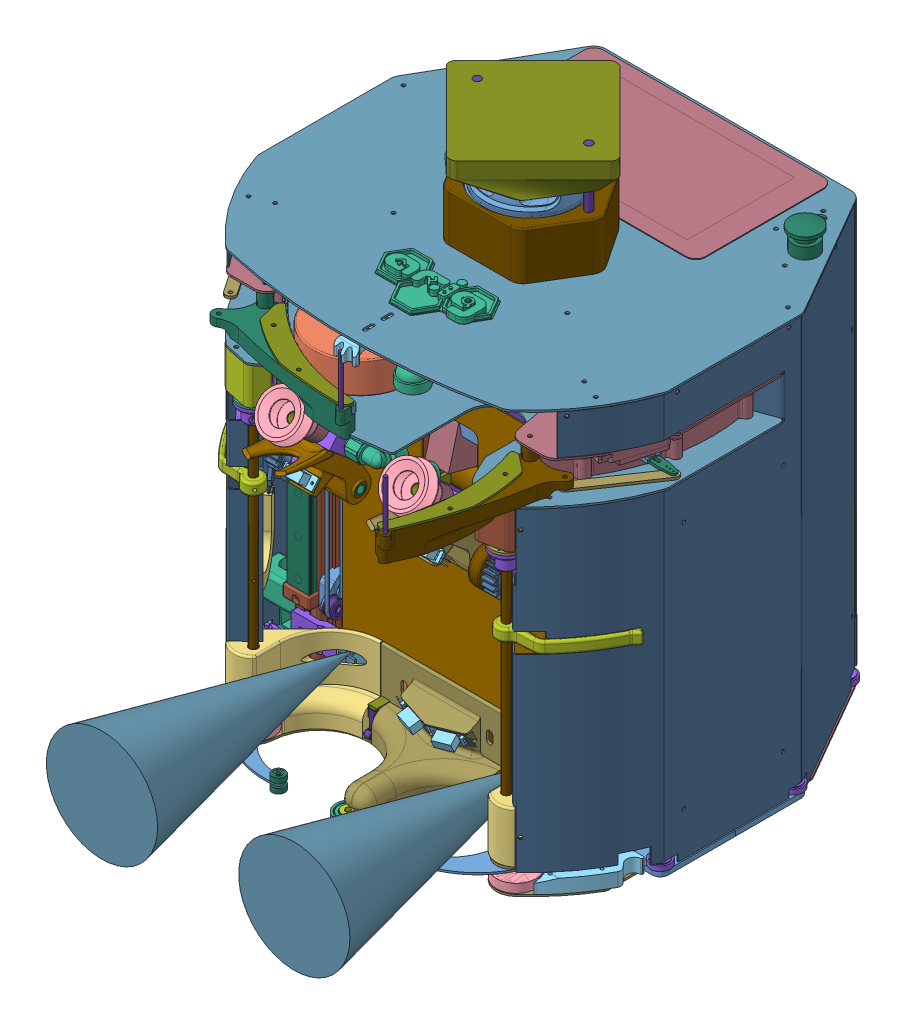
SolidWorks assembly 2019_Gros_robot, configuration Défaut. Lengths in mm. (continued)
Mates (geometry in assembly coordinates): (continued)
- Coaxiale36: concentric anti-aligned: cylinder of roulement-1 through (0 11.5 145.4518) axis (0 1 0) radius 4; cylinder of 20190123-2208-1 through (0 8.1 145.4518) axis (0 -1 0) radius 3.925
- Coïncidente121: coincident anti-aligned: plane of roulement-1 through (2.7957 15 140.7153) normal (0 1 0); plane of 20190123-2208-1 through (5.925 15 145.4518) normal (0 -1 0)
- Coaxiale37: concentric anti-aligned: cylinder of 20190208-2148-1 through (102 235.4 120.9526) axis (0 -1 0) radius 3; cylinder of 20190212-2200-1 through (102 57 120.9526) axis (0 1 0) radius 3.5
- Distance73: distance = 0.8 mm anti-aligned: plane of Roulement_d3xd10xe4-1 through (47.1943 17.95 156.201) normal (0 1 0); plane of 20190208-2207-1 through (102.5 18.75 117.5) normal (0 -1 0)
- Coaxiale39: concentric aligned: cylinder of Roulement_d3xd10xe4-1 through (45.0929 13.95 157.5553) axis (0 -1 0) radius 5; cylinder of 20190208-2207-1 through (45.0929 20.25 157.5553) axis (0 -1 0) radius 1.2
- Tangent1: tangent anti-aligned: cylinder of ? through (50 154.25 120) axis (0 -1 0) radius 38.1; cylinder of Roulement_d3xd10xe4-1 through (49.3866 13.95 163.0956) axis (0 -1 0) radius 5
- Coaxiale42: concentric aligned: cylinder of Roulement_d3xd10xe4-1 through (45.0929 13.95 157.5553) axis (0 -1 0) radius 5; cylinder of Roulement_d3xd10xe4-2 through (45.0929 21.05 157.5553) axis (0 -1 0) radius 5
- Distance74: distance = 0.8 mm anti-aligned: plane of Roulement_d3xd10xe4-2 through (42.6851 21.05 156.8828) normal (0 -1 0); plane of 20190208-2207-1 through (102.5 20.25 117.5) normal (0 1 0)
- Distance80: distance = 50 mm aligned: plane of Palet-1 through (-50 12.7 119.5978) normal (1 0 0); plane of assembly through (0 0 0) normal (1 0 0)
- Coïncidente140: coincident anti-aligned: plane of Robot2019_plaque bille porteuseAvant-1 through (0 7 0) normal (0 1 0); plane of 20190212-2200-1 through (-89.8589 7 116.7694) normal (0 -1 0)
- Coaxiale53: concentric: cylinder of Robot2019_plaque bille porteuseAvant-1 through (-50 7 120) axis (0 -1 0) radius 40; point of 20190212-2200-1
- Parallèle6: parallel anti-aligned: plane of Robot2017_BaseRoulante-1/Robot2015_BaseRoulante_piece01-1 through (0 11 60) normal (0 0 1); plane of 20190212-2200-1 through (-96 29 65) normal (0 0 -1)
- Coïncidente143: coincident anti-aligned: plane of microswitchGaletAss-1/microswitchGalet02-1 through (53.5 29 66) normal (1 0 0); plane of 20190212-2200-1 through (53.5 6.95 144) normal (-1 0 0)
- Coaxiale54: concentric anti-aligned: cylinder of microswitchGaletAss-1/microswitchGalet02-1 through (46.5 14.5 69) axis (1 0 0) radius 1; cylinder of 20190212-2200-1 through (68.5 14.5 69) axis (-1 0 0) radius 1.2
- Coaxiale55: concentric anti-aligned: cylinder of microswitchGaletAss-1/microswitchGalet02-1 through (46.5 23.5 69) axis (1 0 0) radius 1; cylinder of 20190212-2200-1 through (68.5 23.5 69) axis (-1 0 0) radius 1.2
- Coaxiale56: concentric aligned: cylinder of BillePorteuse2019-1 through (105.917 10 116.9526) axis (0 1 0) radius 6.4; cylinder of 20190214-0012-1 through (105.917 4.7 116.9526) axis (0 1 0) radius 8
- Coïncidente144: coincident anti-aligned: plane of BillePorteuse2019-1 through (110.9612 4.7 110.7432) normal (0 1 0); plane of 20190214-0012-1 through (105.917 4.7 116.9526) normal (0 -1 0)
- Coïncidente147: coincident anti-aligned: circle of Servo_HS-85-BB-1; circle of Access_HS-645_BrasRondPetitModele-1
- Coaxiale57: concentric anti-aligned: cylinder of 20190208-2207-1 through (102.5 20.25 117.5) axis (0 -1 0) radius 12; cylinder of Access_HS-645_BrasRondPetitModele-1 through (102.5 24.75 117.5) axis (0 1 0) radius 12
- Coïncidente148: coincident anti-aligned: plane of 20190208-2207-1 through (102.5 20.25 117.5) normal (0 1 0); plane of Access_HS-645_BrasRondPetitModele-1 through (100.0867 20.25 120.3703) normal (0 -1 0)
- Coaxiale58: concentric anti-aligned: cylinder of 20190208-2207-1 through (105.415 18.75 109.5155) axis (0 1 0) radius 1.2; cylinder of Access_HS-645_BrasRondPetitModele-1 through (105.415 30.25 109.5155) axis (0 -1 0) radius 0.5
- Coaxiale59: concentric aligned: cylinder of 20190208-2207-1 through (102.5 20.25 117.5) axis (0 -1 0) radius 12; cylinder of 20190208-2207-2 through (102.5 20.25 117.5) axis (0 -1 0) radius 12
- Angle2: planar angle = 3.185226 rad aligned: plane of 20190208-2207-1 through (102.5 18.75 117.5) normal (-0.572218 0 -0.820101); plane of 20190208-2207-2 through (102.5 18.75 117.5) normal (0.607446 0 0.794361)
- Distance82: distance = 96 mm anti-aligned: plane of Servo_HS-85-BB-1 through (96 25.85 124) normal (-1 0 0); plane of assembly through (0 0 0) normal (1 0 0)
- Distance83: distance = 117.5 mm: point of 20190208-2207-1; plane of assembly
- Distance84: distance = 30 mm aligned: plane of Servo_HS-85-BB-1 through (102.5 37 117.5) normal (0 1 0); plane of Robot2019_plaque bille porteuseAvant-1 through (0 7 0) normal (0 1 0)
- Coaxiale61: concentric aligned: cylinder of Robot2019_plaque bille porteuseAvant-1 through (105.917 7 116.9526) axis (0 -1 0) radius 16; cylinder of 20190214-0012-1 through (105.917 14.7 116.9526) axis (0 -1 0) radius 16
- Coïncidente151: coincident aligned: plane of 20190208-2207-1 through (102.5 20.25 117.5) normal (0 1 0); plane of 20190208-2207-2 through (102.5 20.25 117.5) normal (0 1 0)
- Coaxiale62: concentric aligned: cylinder of Robot2019_plaque bille porteuseAvant-1 through (100.1435 7 126.9526) axis (0 -1 0) radius 1.5; cylinder of 20190214-0012-1 through (100.1435 14.7 126.9526) axis (0 -1 0) radius 1.4
- Coaxiale63: concentric aligned: cylinder of 20181001-2148-1 through (-7.4687 58.1355 42.4725) axis (0.258819 -0.408218 0.875426) radius 0.65; cylinder of 20170416-2304-1/pololu gp2y0d805-1 through (3.2601 41.2137 78.7615) axis (0.258819 -0.408218 0.875426) radius 1
- Coïncidente152: coincident anti-aligned: plane of 20181001-2148-1 through (0 51.0665 85.3479) normal (0.258819 -0.408218 0.875426); plane of 20170416-2304-1/pololu gp2y0d805-1 through (1.0782 36.4945 78.234) normal (-0.258819 0.408218 -0.875426)
- Parallèle7: parallel aligned: plane of 20181001-2148-1 through (1.0353 36.8864 76.4144) normal (0 0.906308 0.422618); plane of 20170416-2304-1/pololu gp2y0d805-1 through (1.4924 43.9981 83.4383) normal (0 0.906308 0.422618)
- Coïncidente157: coincident anti-aligned: plane of Robot2019_plaque bille porteuseAvant-1 through (0 7 0) normal (0 1 0); plane of 20190219-0006-1 through (105.917 7 116.9526) normal (0 -1 0)
- Coaxiale64: concentric aligned: cylinder of Robot2019_plaque bille porteuseAvant-1 through (0 7 0) axis (0 -1 0) radius 173.7857; cylinder of 20190219-0006-1 through (0 18 0) axis (0 -1 0) radius 174
- Coïncidente158: coincident aligned: plane of 20190219-0006-1 through (0 7 0) normal (0 0 1); plane of assembly through (0 0 0) normal (0 0 1)
- Coïncidente159: coincident aligned: plane of Roulement_d3xd10xe4-1 through (47.1943 13.95 156.201) normal (0 -1 0); plane of Roulement_d3xd10xe4-3 through (160.2067 13.95 73.6245) normal (0 -1 0)
- Coaxiale65: concentric aligned: cylinder of 20190208-2207-2 through (158.1053 20.25 74.9788) axis (0 -1 0) radius 4; cylinder of Roulement_d3xd10xe4-3 through (158.1053 13.95 74.9788) axis (0 -1 0) radius 5
- Coïncidente161: coincident anti-aligned: plane of 20190219-0101-1 through (130 61.0678 59) normal (-1 0 0); plane of Robot2019_profiléX20_02-3 through (130 11 46.7) normal (1 0 0)
- Distance86: distance = 1 mm aligned: plane of 20190219-0101-1 through (130 61.0678 59) normal (0 0 1); plane of Robot2019_profiléX20_02-3 through (123.3 11 60) normal (0 0 1)
- Coïncidente162: coincident aligned: plane of 20190219-0101-1 through (163 14.6933 37) normal (1 0 0); plane of 20190219-0101-2 through (163 87.4423 -37) normal (1 0 0)
- Coïncidente163: coincident aligned: plane of 20190219-0101-1 through (130 61.0678 50) normal (0 1 0); plane of 20190219-0101-2 through (130 61.0678 -50) normal (0 1 0)
- Distance87: distance = 1 mm aligned: plane of 20190219-0101-2 through (130 41.0678 -59) normal (0 0 -1); plane of Robot2019_profiléX20_02-4 through (128 11 -60) normal (0 0 -1)
- Coaxiale66: concentric aligned: cylinder of 20190208-2148-1 through (102 235.4 120.9526) axis (0 -1 0) radius 3; cylinder of 20190220-2148-1 through (102 186.4 120.9526) axis (0 -1 0) radius 3.1
- Coaxiale67: concentric aligned: cylinder of Servo_HS-85-BB-2 through (102 241.9 120.9526) axis (0 1 0) radius 2.75; cylinder of Access_HS-645_BrasRondPetitModele-2 through (102 244.9 120.9526) axis (0 1 0) radius 2.75
- Coïncidente164: coincident anti-aligned: plane of Servo_HS-85-BB-2 through (102 241.9 120.9526) normal (0 -1 0); plane of Access_HS-645_BrasRondPetitModele-2 through (99.4128 241.9 121.8847) normal (0 1 0)
- Coïncidente165: coincident anti-aligned: plane of Robot2019_plaque du dessus-1 through (0 276 -355) normal (0 -1 0); plane of Servo_HS-85-BB-2 through (102 276 120.9526) normal (0 1 0)
- Coaxiale68: concentric anti-aligned: cylinder of 20190208-2148-1 through (102 235.4 120.9526) axis (0 -1 0) radius 3; cylinder of Access_HS-645_BrasRondPetitModele-2 through (102 244.9 120.9526) axis (0 1 0) radius 12
- Coaxiale70: concentric aligned: cylinder of Access_HS-645_BrasRondPetitModele-2 through (102 244.9 120.9526) axis (0 1 0) radius 12; cylinder of 20190221-0033-1 through (102 240.4 120.9526) axis (0 1 0) radius 12
- Coïncidente168: coincident anti-aligned: plane of Access_HS-645_BrasRondPetitModele-2 through (98.472 240.4 122.2237) normal (0 -1 0); plane of 20190221-0033-1 through (99.4389 240.4 117.88) normal (0 1 0)
- Coaxiale71: concentric anti-aligned: cylinder of Access_HS-645_BrasRondPetitModele-2 through (95.5972 250.4 113.2712) axis (0 -1 0) radius 0.5; cylinder of 20190221-0033-1 through (95.5972 225.4 113.2712) axis (0 1 0) radius 1.2
- Distance91: distance = 4 mm aligned: plane of Raspberry pi3 Screen assembly-1 through (-9.296 346 -101.85) normal (0 1 0); plane of assembly through (0 350 0) normal (0 1 0)
- Coaxiale72: concentric aligned: cylinder of 20190208-2148-1 through (99.6956 229.4 122.8734) axis (0.768138 0 -0.640285) radius 1.25; cylinder of 20190221-0033-1 through (92.7823 229.4 128.636) axis (0.768138 0 -0.640285) radius 1.5
- Coaxiale73: concentric aligned: cylinder of 20190208-2148-1 through (99.6956 181.4 122.8734) axis (0.768138 0 -0.640285) radius 1.25; cylinder of 20190220-2148-1 through (108.1451 181.4 115.8303) axis (0.768138 0 -0.640285) radius 1.2
- AngleLimite1: limit planar angle = 0.418879 rad aligned: plane of 20190220-2148-1 through (102 181.4 120.9526) normal (0.913545 0 0.406737); plane of assembly through (0 0 0) normal (1 0 0)
- Coïncidente169: coincident aligned: plane of Carter2019-1 through (0 7 0) normal (0 0 1); plane of assembly through (0 0 0) normal (0 0 1)
- Coïncidente170: coincident aligned: plane of Carter2019-1 through (0 7 0) normal (1 0 0); plane of assembly through (0 0 0) normal (1 0 0)
- Coïncidente171: coincident anti-aligned: plane of Robot2017_BaseRoulante-1/Robot2015_BaseRoulante_piece01-1 through (0 7 0) normal (0 -1 0); plane of Carter2019-1 through (0 7 0) normal (0 1 0)
- Coïncidente172: coincident anti-aligned: plane of Robot2019_plaque du dessus-1 through (0 276 -355) normal (0 -1 0); plane of 20190223-1730-1 through (-0.1299 276 -354.8724) normal (0 1 0)
- Coïncidente173: coincident anti-aligned: plane of Servo_HS-85-BB-2 through (124.7356 246 115.3317) normal (0.5 0 0.866025); plane of 20190223-1730-1 through (125.0387 276 115.1567) normal (-0.5 0 -0.866025)
- Coaxiale75: concentric aligned: cylinder of Servo_HS-85-BB-2 through (93.6429 257.15 125.7776) axis (0 -1 0) radius 1.5; cylinder of 20190223-1730-1 through (93.6429 276 125.7776) axis (0 -1 0) radius 1.2
- Parallèle9: parallel aligned: plane of assembly through (0 0 0) normal (1 0 0); plane of 20190223-1730-1 through (-0.1299 256 0.1276) normal (1 0 0)
- Coaxiale76: concentric aligned: cylinder of 20181002-0030-1/20181002-0031-4 through (0 293.5 0) axis (0 -1 0) radius 141; cylinder of 20181002-0216-1/20181002-0217-1 through (0 296.5 0) axis (0 -1 0) radius 141
- Coïncidente175: coincident anti-aligned: plane of 20181001-2148-1 through (0 51.0665 85.3479) normal (-0.258819 -0.408218 0.875426); plane of 20170416-2304-2/pololu gp2y0d805-1 through (-1.0782 44.6512 82.0376) normal (0.258819 0.408218 -0.875426)
- Coaxiale77: concentric aligned: cylinder of 20181001-2148-1 through (7.4687 58.1355 42.4725) axis (-0.258819 -0.408218 0.875426) radius 0.65; cylinder of 20170416-2304-2/pololu gp2y0d805-1 through (-3.2601 41.2137 78.7615) axis (-0.258819 -0.408218 0.875426) radius 1
- Parallèle10: parallel aligned: plane of 20181001-2148-1 through (1.0353 36.8864 76.4144) normal (0 0.906308 0.422618); plane of 20170416-2304-2/pololu gp2y0d805-1 through (-1.4924 43.9981 83.4383) normal (0 0.906308 0.422618)
- Coaxiale78: concentric aligned: cylinder of Robot2019_plaque du dessus-1 through (0 267.5 0) axis (0 1 0) radius 27; cylinder of 20190221-0152-1 through (0 274.2 0) axis (0 1 0) radius 25.3
- Distance94: distance = 1.5 mm anti-aligned: plane of 20190221-0152-1 through (0 311 0) normal (0 -1 0); plane of 20181002-0030-1/20181002-0031-2 through (0 309.5 0) normal (0 1 0)
- Coïncidente177: coincident anti-aligned: plane of 20190221-0152-1; plane of assembly through (0 0 0) normal (1 0 0)
- Coïncidente178: coincident anti-aligned: plane of Symétrie20181002-0216-3/Symétrie20181002-0217-1 through (136.9152 290.5 112.3728) normal (0 -1 0); plane of 20190225-2214-1 through (134.7726 290.5 106.5984) normal (0 1 0)
- Coaxiale79: concentric aligned: cylinder of Symétrie20181002-0216-3/Symétrie20181002-0217-1 through (134.7726 430.1481 106.5984) axis (0 -1 0) radius 1.5; cylinder of 20190225-2214-1 through (134.7726 290.5 106.5984) axis (0 -1 0) radius 1.5
- Coaxiale80: concentric anti-aligned: cylinder of Access_HS-485_BrasReglablePartieB-1 through (170.1591 290.05 54.4756) axis (0 1 0) radius 0.5; cylinder of 20190225-2214-1 through (170.1591 290.5 54.4756) axis (0 -1 0) radius 1.5
- Coïncidente179: coincident anti-aligned: plane of 20181002-0030-1/20181002-0031-2 through (0 309.5 0) normal (0 1 0); plane of Robot2019_plaque elec-1 through (0 309.5 -355) normal (0 -1 0)
- Coaxiale83: concentric anti-aligned: cylinder of Robot2019_plaque elec-1 through (143 301 86.913) axis (0 1 0) radius 1.5; cylinder of Servo_HS-485-HB-1 through (143 309.5 86.913) axis (0 -1 0) radius 1.5
- Parallèle13: parallel aligned: plane of Servo_HS-485-HB-1 through (159.9911 312.35 48.1691) normal (0.95652 0 0.291667); plane of Robot2019_plaque elec-1 through (141.4855 301 40.4511) normal (0.95652 0 0.291667)
- AngleLimite2: limit planar angle = 1.140703 rad anti-aligned: plane of Robot2019_plaque du dessus-1 through (30 275.999 141.0123) normal (0.130526 0 0.991445); plane of Symétrie20181002-0216-3/Symétrie20181002-0217-1 through (97.146 243.6998 219.4091) normal (-0.955574 0 -0.29475)
- Distance95: distance = 5 mm aligned: plane of Robot2019_plaque superieure-2 through (0 345 -355) normal (0 1 0); plane of assembly through (0 350 0) normal (0 1 0)
- Coïncidente185: coincident anti-aligned: plane of rplidar-a2-1 through (0 362.5 0) normal (0 -1 0); plane of 20161105-0900-1 through (0 362.5 0) normal (0 1 0)
- Coaxiale85: concentric anti-aligned: cylinder of rplidar-a2-1 through (-20.8597 362.5 20.8597) axis (0 1 0) radius 1.6; cylinder of 20161105-0900-1 through (-20.8597 380.5 20.8597) axis (0 -1 0) radius 1.5
- Coaxiale86: concentric anti-aligned: cylinder of rplidar-a2-1 through (-20.8597 362.5 -20.8597) axis (0 1 0) radius 1.6; cylinder of 20161105-0900-1 through (-20.8597 380.5 -20.8597) axis (0 -1 0) radius 1.5
- Coaxiale87: concentric aligned: cylinder of 20161105-0900-1 through (-45 380.5 -2.5) axis (0 -1 0) radius 3; cylinder of 20161106-1538-1 through (-45 430 -2.5) axis (0 -1 0) radius 3
- Coaxiale88: concentric aligned: cylinder of 20190313-2117-1 through (-45 430 -2.5) axis (0 -1 0) radius 3.1; cylinder of 20161106-1538-1 through (-45 430 -2.5) axis (0 -1 0) radius 3
- Coaxiale89: concentric aligned: cylinder of 20161105-0900-1 through (45 380.5 -2.5) axis (0 -1 0) radius 3; cylinder of 20161106-1538-2 through (45 430 -2.5) axis (0 -1 0) radius 3
- Coaxiale90: concentric aligned: cylinder of 20190313-2117-1 through (45 430 -2.5) axis (0 -1 0) radius 3.1; cylinder of 20161106-1538-2 through (45 430 -2.5) axis (0 -1 0) radius 3
- Coïncidente186: coincident aligned: plane of 20190313-2117-1 through (0 430 -2.5) normal (0 1 0); plane of 20161106-1538-2 through (45 430 -2.5) normal (0 1 0)
- Coïncidente187: coincident aligned: plane of 20190313-2117-1 through (0 430 -2.5) normal (0 1 0); plane of 20161106-1538-1 through (-45 430 -2.5) normal (0 1 0)
- Coïncidente188: coincident anti-aligned: plane of Robot2019_plaque superieure-2 through (0 345 -355) normal (0 1 0); plane of 20161105-0900-1 through (45 345 -2.5) normal (0 -1 0)
- Coïncidente189: coincident aligned: plane of 20190313-2117-1 through (0 430 -2.5) normal (0 1 0); plane of assembly through (0 430 0) normal (0 1 0)
- Coïncidente190: coincident aligned: plane of 20161105-0900-1 through (0 345 0) normal (0 0 1); plane of assembly through (0 0 0) normal (0 0 1)
- Coïncidente191: coincident aligned: plane of 20161105-0900-1 through (0 345 0) normal (1 0 0); plane of assembly through (0 0 0) normal (1 0 0)
- Distance96: distance = 1 mm anti-aligned: plane of Robot2019_plaque superieure-2 through (76.184 342 -152) normal (-1 0 0); plane of Raspberry pi3 Screen assembly-1 through (75.184 340.04 -50) normal (1 0 0)
- Distance97: distance = 2 mm aligned: plane of 20170416-2304-3/SupportCapteurPololu-1 through (-128 238.5 -30) normal (-1 0 0); plane of Robot2019_profiléX20_02-2 through (-130 11 -46.7) normal (-1 0 0)
- Distance98: distance = 40 mm aligned: plane of 20170416-2304-3/SupportCapteurPololu-1 through (-120 226 0) normal (0 0 1); plane of Robot2019_profiléX20_02-2 through (-128 11 -40) normal (0 0 1)
- Distance99: distance = 50 mm aligned: plane of 20170416-2304-3/SupportCapteurPololu-1 through (-128 226 -30) normal (0 -1 0); plane of Robot2019_plaque du dessus-1 through (0 276 -355) normal (0 -1 0)
- Distance100: distance = 3 mm anti-aligned: plane of Adafruit_TCS34725-1 through (-106.6 273 31) normal (0 1 0); plane of Robot2019_plaque du dessus-1 through (0 276 -355) normal (0 -1 0)
- Distance102: distance = 9 mm anti-aligned: plane of Adafruit_TCS34725-1 through (-106.6 269 31) normal (0 0 1); plane of Robot2019_profiléX20_02-1 through (-123.3 11 40) normal (0 0 -1)
- Distance103: distance = 3 mm aligned: plane of Robot2019_profiléX20_02-1 through (-130 11 42) normal (-1 0 0); plane of Adafruit_TCS34725-1 through (-127 269 31) normal (-1 0 0)
- Coïncidente199: coincident anti-aligned: plane of Robot2019_profiléX20_02-1 through (-123.3 11 40) normal (0 0 -1); plane of 20190227-2336-1 through (-122.35 269 40) normal (0 0 1)
- Distance104: distance = 1.5 mm aligned: plane of 20190227-2336-1 through (-128.5 269 37) normal (-1 0 0); plane of Robot2019_profiléX20_02-1 through (-130 11 42) normal (-1 0 0)
- Coïncidente201: coincident anti-aligned: plane of Adafruit_TCS34725-1 through (-106.6 269 31) normal (0 -1 0); plane of 20190227-2336-1 through (-120 269 40) normal (0 1 0)
- Coïncidente205: coincident anti-aligned: plane of Robot2019_profiléX20_02-1 through (-112 11 40) normal (0 0 -1); plane of 20190228-0009-1 through (-147.0576 165.5788 40) normal (0 0 1)
- Coïncidente206: coincident anti-aligned: plane of 20190228-0009-1 through (0 165.5788 39.25) normal (-1 0 0); plane of assembly through (0 0 0) normal (1 0 0)
- Coïncidente207: coincident anti-aligned: plane of 20181005-1508-1/20181006-0057-1 through (-48 165.5788 10.194) normal (0 -1 0); plane of 20190228-0009-1 through (-127.5 165.5788 49) normal (0 1 0)
- Coïncidente208: coincident anti-aligned: plane of 20181005-1508-1/Servo_HS-485-HB-1 through (-34 207.5 -31.6025) normal (1 0 0); plane of Robot2015_supportServo02-1 through (-34 217.5 -3.6025) normal (-1 0 0)
- Coaxiale91: concentric aligned: cylinder of 20181005-1508-1/20181006-0057-1 through (-39 241.5 -36.6025) axis (-1 0 0) radius 1.2; cylinder of Robot2015_supportServo02-1 through (-32.5 241.5 -36.6025) axis (-1 0 0) radius 1.5
- Coaxiale92: concentric aligned: cylinder of 20181005-1508-1/20181006-0057-1 through (-39 241.5 -26.6025) axis (-1 0 0) radius 1.2; cylinder of Robot2015_supportServo02-1 through (-32.5 241.5 -26.6025) axis (-1 0 0) radius 1.5
- Coïncidente209: coincident aligned: plane of Robot2019_plaque superieure-2 through (0 343.5 0) normal (0 0 1); plane of assembly through (0 0 0) normal (0 0 1)
- Coïncidente210: coincident aligned: plane of Robot2019_plaque superieure-2 through (0 343.5 0) normal (1 0 0); plane of assembly through (0 0 0) normal (1 0 0)
- Coaxiale93: concentric anti-aligned: cylinder of APEM_A01ES_A0154B-1 through (121.8383 364 -100) axis (0 -1 0) radius 8; cylinder of Robot2019_plaque superieure-2 through (121.8383 342 -100) axis (0 1 0) radius 8
- Coïncidente211: coincident anti-aligned: plane of APEM_A01ES_A0154B-1 through (126.8383 345 -91.3397) normal (0 -1 0); plane of Robot2019_plaque superieure-2 through (0 345 -355) normal (0 1 0)
- Coïncidente212: coincident anti-aligned: plane of Raspberry pi3 Screen assembly-1 through (-7.916 340.04 -100.3) normal (0 -1 0); plane of 20190301-2106-1 through (47.184 340.04 -143.825) normal (0 1 0)
- Coaxiale94: concentric anti-aligned: cylinder of Raspberry pi3 Screen assembly-1 through (55.184 340.04 -135.65) axis (0 -1 0) radius 1.5; cylinder of 20190301-2106-1 through (55.184 335.04 -135.65) axis (0 1 0) radius 1.5
- Parallèle14: parallel aligned: plane of Raspberry pi3 Screen assembly-1 through (75.184 340.04 -150.6) normal (0 0 -1); plane of 20190301-2106-1 through (47.184 337.04 -143.825) normal (0 0 -1)
- Coïncidente214: coincident anti-aligned: plane of Robot2019_plaque superieure-2 through (0 343.5 -355) normal (0 -1 0); plane of 20190301-2139-1 through (0 343.5 115) normal (0 1 0)
- Coïncidente215: coincident aligned: plane of 20190301-2139-1 through (0 343.5 0) normal (1 0 0); plane of assembly through (0 0 0) normal (1 0 0)
- Coïncidente216: coincident aligned: plane of 20190301-2139-1 through (0 343.5 0) normal (0 0 1); plane of assembly through (0 0 0) normal (0 0 1)
- Coïncidente217: coincident aligned: plane of Robot2019_plaque elec-1 through (0 309.5 0) normal (0 0 1); plane of assembly through (0 0 0) normal (0 0 1)
- Coïncidente218: coincident aligned: plane of Robot2019_plaque elec-1 through (0 309.5 0) normal (1 0 0); plane of assembly through (0 0 0) normal (1 0 0)
- Coïncidente219: coincident aligned: plane of Robot2019_plaque du dessus-1 through (0 276 0) normal (0 0 1); plane of assembly through (0 0 0) normal (0 0 1)
- Coaxiale95: concentric anti-aligned: cylinder of Robot2019_plaque superieure-2 through (30 343.5 80) axis (0 1 0) radius 1.5; cylinder of LogoARIG2-1 through (30 353.3941 80) axis (0 -1 0) radius 1.2
- Coaxiale96: concentric anti-aligned: cylinder of Robot2019_plaque superieure-2 through (-30 343.5 80) axis (0 1 0) radius 1.5; cylinder of LogoARIG2-1 through (-30 353.3941 80) axis (0 -1 0) radius 1.2
- Coïncidente220: coincident anti-aligned: plane of Robot2019_plaque superieure-2 through (0 345 -355) normal (0 1 0); plane of LogoARIG2-1 through (-42.5 345 104) normal (0 -1 0)
- Coaxiale99: concentric aligned: cylinder of Robot2019_plaque du dessus-1 through (56.5 275.999 -145) axis (0 1 0) radius 1.25; cylinder of GP2D-2 through (56.5 277.5 -145) axis (0 1 0) radius 1.6
- Coaxiale100: concentric aligned: cylinder of Robot2019_plaque du dessus-1 through (93.5 275.999 -145) axis (0 1 0) radius 1.25; cylinder of GP2D-2 through (93.5 277.5 -145) axis (0 1 0) radius 1.6
- Coïncidente223: coincident anti-aligned: plane of Raspberry pi3 Screen assembly-1 through (-91.016 340.04 -50) normal (0 0 1); plane of Robot2019_plaque superieure-2 through (5.7325 342 -50) normal (0 0 -1)
- Coïncidente224: coincident anti-aligned: plane of 20181006-0254-1 through (-106.5 343.5 -156.0025) normal (0 1 0); plane of Robot2019_plaque superieure-2 through (0 343.5 -355) normal (0 -1 0)
- Coaxiale101: concentric anti-aligned: cylinder of Raspberry pi3 Screen assembly-1 through (-71.016 340.04 -135.65) axis (0 -1 0) radius 1.5; cylinder of 20190301-2106-2 through (-71.016 335.04 -135.65) axis (0 1 0) radius 1.5
- Coaxiale102: concentric anti-aligned: cylinder of Raspberry pi3 Screen assembly-1 through (-71.016 340.04 -70) axis (0 -1 0) radius 1.5; cylinder of 20190301-2106-2 through (-71.016 335.04 -70) axis (0 1 0) radius 1.5
- Coïncidente225: coincident anti-aligned: plane of Raspberry pi3 Screen assembly-1 through (-7.916 340.04 -100.3) normal (0 -1 0); plane of 20190301-2106-2 through (-63.016 340.04 -61.825) normal (0 1 0)
- Coaxiale103: concentric anti-aligned: cylinder of 20181006-0254-1 through (-30 268.5 -156.0025) axis (0 0 -1) radius 1.5; cylinder of LogoARIG2-2 through (-30 268.5 -168.3967) axis (0 0 1) radius 1.2
- Coaxiale104: concentric anti-aligned: cylinder of 20181006-0254-1 through (30 268.5 -156.0025) axis (0 0 -1) radius 1.5; cylinder of LogoARIG2-2 through (30 268.5 -168.3967) axis (0 0 1) radius 1.2
- Coïncidente226: coincident anti-aligned: plane of 20181006-0254-1 through (0 343.5 -160.0025) normal (0 0 -1); plane of LogoARIG2-2 through (42.5 244.5 -160.0025) normal (0 0 1)
- Coïncidente227: coincident anti-aligned: plane of Robot2019_plaque superieure-2 through (0 343.5 -355) normal (0 -1 0); plane of 20190308-1510-1 through (0 343.5 0) normal (0 1 0)
- Coïncidente228: coincident aligned: plane of 20190308-1510-1 through (0 336.5 0) normal (0 0 1); plane of assembly through (0 0 0) normal (0 0 1)
- Coïncidente229: coincident aligned: plane of 20190308-1510-1 through (0 336.5 0) normal (1 0 0); plane of assembly through (0 0 0) normal (1 0 0)
- Coïncidente232: coincident anti-aligned: plane of Robot2019_plaque superieure-2 through (0 343.5 -355) normal (0 -1 0); plane of 20190308-2149-1 through (0 343.5 0) normal (0 1 0)
- Coaxiale105: concentric anti-aligned: cylinder of Robot2019_plaque superieure-2 through (-155 342 -53) axis (0 1 0) radius 1.5; cylinder of 20190308-2149-1 through (-155 354.8137 -53) axis (0 -1 0) radius 1.2
- Coaxiale106: concentric anti-aligned: cylinder of Robot2019_plaque superieure-2 through (-140 342 87) axis (0 1 0) radius 1.5; cylinder of 20190308-2149-1 through (-140 354.8137 87) axis (0 -1 0) radius 1.2
- Coïncidente233: coincident anti-aligned: line of 20190308-1510-1 through (152.4215 312 -59.2282) axis (-0.5 0 -0.866025); line of interrupteur principal-1 through (137.9215 312 -84.3429) axis (0.5 0 0.866025)
- Coïncidente234: coincident anti-aligned: line of 20190308-1510-1 through (137.9215 312 -84.3429) axis (0 1 0); line of interrupteur principal-1 through (137.9215 334 -84.3429) axis (0 -1 0)
- Coïncidente235: coincident anti-aligned: plane of Robot2019_plaque elec-1 through (0 311 -355) normal (0 1 0); plane of 20190309-0049-1 through (-60 311 83) normal (0 -1 0)
- Coaxiale107: concentric anti-aligned: cylinder of Robot2019_plaque elec-1 through (-70 309.5 40) axis (0 1 0) radius 1.5; cylinder of 20190309-0049-1 through (-70 354.3137 40) axis (0 -1 0) radius 1.2
- Coaxiale108: concentric anti-aligned: cylinder of Robot2019_plaque elec-1 through (70 309.5 40) axis (0 1 0) radius 1.5; cylinder of 20190309-0049-1 through (70 354.3137 40) axis (0 -1 0) radius 1.2
- Coïncidente236: coincident anti-aligned: plane of Robot2019_profiléX20_02-1 through (-130 11 53.3) normal (-1 0 0); plane of 20190309-0127_Corniere_15.5x27.5x1.5-1 through (-130 260.5 59) normal (1 0 0)
- Distance106: distance = 1 mm aligned: plane of Robot2019_profiléX20_02-1 through (-128 11 60) normal (0 0 1); plane of 20190309-0127_Corniere_15.5x27.5x1.5-1 through (-130 276 59) normal (0 0 1)
- Coïncidente238: coincident anti-aligned: plane of Robot2019_plaque du dessus-1 through (0 276 -355) normal (0 -1 0); plane of 20190309-0127_Corniere_15.5x27.5x1.5-1 through (-130 276 59) normal (0 1 0)
- Coïncidente242: coincident anti-aligned: plane of 20181006-0254-1 through (0 343.5 -156.0025) normal (0 0 1); plane of Ventilo-2 through (75 318.5 -156.0025) normal (0 0 -1)
- Coaxiale109: concentric aligned: cylinder of 20181006-0254-1 through (91 302.5 -156.0025) axis (0 0 -1) radius 1.5; cylinder of Ventilo-2 through (91 302.5 -146.0025) axis (0 0 -1) radius 1.5
- Coaxiale110: concentric aligned: cylinder of 20181006-0254-1 through (59 334.5 -156.0025) axis (0 0 -1) radius 1.5; cylinder of Ventilo-2 through (59 334.5 -146.0025) axis (0 0 -1) radius 1.5
- Distance107: distance = 10 mm aligned: plane of GP2D-2 through (56.5 287.5 -145) normal (0 1 0); plane of Robot2019_plaque du dessus-1 through (0 277.5 -355) normal (0 1 0)
- Coïncidente245: coincident anti-aligned: plane of TelemetreTOF_RB-Mce-01-1 through (-74.5065 272.4886 -143) normal (-0.139173 0.990268 0); plane of 20190314-1109-1 through (-74.5065 272.4886 -143) normal (0.139173 -0.990268 0)
- Coaxiale111: concentric anti-aligned: cylinder of TelemetreTOF_RB-Mce-01-1 through (-74.2977 271.0032 -133) axis (-0.139173 0.990268 0) radius 1; cylinder of 20190314-1109-1 through (-75.8982 282.3912 -133) axis (0.139173 -0.990268 0) radius 1.5
- Coaxiale112: concentric anti-aligned: cylinder of TelemetreTOF_RB-Mce-01-1 through (-74.2977 271.0032 -153) axis (-0.139173 0.990268 0) radius 1; cylinder of 20190314-1109-1 through (-75.8982 282.3912 -153) axis (0.139173 -0.990268 0) radius 1.5
- Coïncidente246: coincident anti-aligned: plane of Robot2019_plaque du dessus-1 through (0 276 -355) normal (0 -1 0); plane of 20190314-1109-1 through (-84.0884 276 -143) normal (0 1 0)
- Coaxiale113: concentric: cylinder of Robot2019_plaque du dessus-1 through (-75 276 -133) axis (0 1 0) radius 1.5; point of 20190314-1109-1
- Parallèle15: parallel aligned: plane of 20181006-0254-1 through (0 343.5 -160.0025) normal (0 0 -1); plane of 20190314-1109-1 through (-84.8106 281.1387 -155.5) normal (0 0 -1)
- Coïncidente247: coincident anti-aligned: plane of 20181005-1508-1/20181005-2259-1 through (50 7 -156.0025) normal (0 0 -1); plane of 20181006-0254-1 through (0 343.5 -156.0025) normal (0 0 1)
- Coïncidente248: coincident anti-aligned: plane of 20181005-1508-1/20181005-2259-1 through (-50 7 -156.0025) normal (0 0 -1); plane of 20181006-0255-1 through (0 133.2 -156.0025) normal (0 0 1)
- Coaxiale114: concentric aligned: cylinder of 20181006-0254-1 through (-100.4378 343.5 -153.5025) axis (0 1 0) radius 6.5; cylinder of 20181006-0255-1 through (-100.4378 133.2 -153.5025) axis (0 1 0) radius 6.5
- Coaxiale115: concentric aligned: cylinder of 20181005-1508-1/20181005-2259-1 through (0 93.2 -141.0025) axis (0 0 -1) radius 1.2; cylinder of 20181006-0255-1 through (0 93.2 -156.0025) axis (0 0 -1) radius 1.5
- Coïncidente249: coincident anti-aligned: plane of 20181006-0255-1 through (10.5 53.2 -156.5025) normal (0 0 1); plane of Palet-2 through (51.9 38.1 -156.5025) normal (0 0 -1)
- Distance108: distance = 50 mm anti-aligned: plane of Palet-2 through (50 38.1 -143.8025) normal (-1 0 0); plane of assembly through (0 0 0) normal (1 0 0)
- Tangent2: tangent anti-aligned: cylinder of Palet-2 through (51.9 38.1 -156.5025) axis (0 0 1) radius 38.1; plane of assembly through (0 0 0) normal (0 1 0)
- Tangent3: tangent anti-aligned: plane of 20181005-1508-1/20181005-2259-1 through (90 156.9313 499843.9975) normal (-1 0 0); cylinder of Palet-2 through (51.9 38.1 -156.5025) axis (0 0 1) radius 38.1
- Coaxiale116: concentric anti-aligned: cylinder of TelemetreTOF_RB-Mce-01-2 through (87.5 42 66) axis (0 0 -1) radius 1; cylinder of 20190331-1440-1 through (87.5 42 60) axis (0 0 1) radius 1.5
- Coaxiale117: concentric anti-aligned: cylinder of TelemetreTOF_RB-Mce-01-2 through (67.5 42 66) axis (0 0 -1) radius 1; cylinder of 20190331-1440-1 through (67.5 42 60) axis (0 0 1) radius 1.5
- Coïncidente250: coincident anti-aligned: plane of TelemetreTOF_RB-Mce-01-2 through (77.5 42 64.5) normal (0 0 -1); plane of 20190331-1440-1 through (77.5 42 64.5) normal (0 0 1)
- Coïncidente251: coincident anti-aligned: plane of Robot2019_profiléX20_02-3 through (112 11 60) normal (0 0 1); plane of 20190331-1440-1 through (77.5 42 60) normal (0 0 -1)
- Distance109: distance = 2 mm aligned: plane of 20190331-1440-1 through (128 31 106.1203) normal (1 0 0); plane of Robot2019_profiléX20_02-3 through (130 11 58) normal (1 0 0)
- Distance110: distance = 20 mm anti-aligned: plane of 20190331-1440-1 through (92.5 31 60) normal (0 -1 0); plane of Robot2017_BaseRoulante-1/Robot2015_BaseRoulante_piece01-1 through (0 11 0) normal (0 1 0)
- Coïncidente254: coincident anti-aligned: plane of 20161105-0900-1 through (0 380.5 0) normal (0 1 0); plane of 20190331-1545-1 through (0 380.5 0) normal (0 -1 0)
- Coaxiale118: concentric anti-aligned: cylinder of 20161106-1538-1 through (-45 430 -2.5) axis (0 -1 0) radius 3; cylinder of 20190331-1545-1 through (-45 380.5 -2.5) axis (0 1 0) radius 3
- Coaxiale119: concentric anti-aligned: cylinder of 20161106-1538-2 through (45 430 -2.5) axis (0 -1 0) radius 3; cylinder of 20190331-1545-1 through (45 380.5 -2.5) axis (0 1 0) radius 3
- Coaxiale120: concentric anti-aligned: cylinder of 20180929-0119-1/12v-silent-dc-motor-146rpm-encoder-desc-dime-1 through (-9.8995 248.4645 12.6005) axis (0 1 0) radius 1.25; cylinder of 20190331-1640-1 through (-9.8995 260 12.6005) axis (0 -1 0) radius 1.5
- Coaxiale121: concentric anti-aligned: cylinder of 20180929-0119-1/12v-silent-dc-motor-146rpm-encoder-desc-dime-1 through (-9.8995 248.4645 32.3995) axis (0 1 0) radius 1.25; cylinder of 20190331-1640-1 through (-9.8995 260 32.3995) axis (0 -1 0) radius 1.5
- Coïncidente255: coincident anti-aligned: plane of 20180929-0119-1/12v-silent-dc-motor-146rpm-encoder-desc-dime-1 through (12.7279 257 9.7721) normal (0 1 0); plane of 20190331-1640-1 through (0 257 22.5) normal (0 -1 0)
- Parallèle18: parallel aligned: plane of 20181005-1508-1/20181006-0057-1 through (-48 251 27.3975) normal (0 0 1); plane of 20190331-1640-1 through (-45 222 45.5) normal (0 0 1)
- Coaxiale122: concentric aligned: cylinder of 20190309-0127_Corniere_15.5x27.5x1.5-1 through (-145.7716 272 28.3351) axis (0 1 0) radius 1.5; cylinder of 20190309-0128-1 through (-145.7716 260.5 28.3351) axis (0 1 0) radius 1.5
- Coaxiale123: concentric aligned: cylinder of 20190309-0127_Corniere_15.5x27.5x1.5-1 through (-134 267 50) axis (1 0 0) radius 2.5; cylinder of 20190309-0128-1 through (-157.5 267 50) axis (1 0 0) radius 5
- Coaxiale124: concentric aligned: cylinder of 20170416-2304-3/pololu gp2y0d805-1 through (-120 235.9 -3) axis (0 1 0) radius 1; cylinder of SupportCapteurPololuSpecial2019-1 through (-120 226 -3) axis (0 1 0) radius 0.75
- Parallèle19: parallel aligned: plane of 20170416-2304-3/pololu gp2y0d805-1 through (-115.5 238.4 -0.5) normal (0 0 1); plane of SupportCapteurPololuSpecial2019-1 through (-120 226 0) normal (0 0 1)
- Coïncidente257: coincident anti-aligned: plane of 20170416-2304-3/pololu gp2y0d805-1 through (-115.5 236.8 -0.5) normal (0 -1 0); plane of SupportCapteurPololuSpecial2019-1 through (-120 236.8 -15) normal (0 1 0)
- Coïncidente258: coincident anti-aligned: plane of Robot2017_BaseRoulante-1/Robot2015_profiléX20_01-1 through (-46 176 -60) normal (0 0 -1); plane of Robot2015_BaseRoulante_piece15-1 through (95 119.5 -60) normal (0 0 1)
- Distance111: distance = 70 mm aligned: plane of Robot2015_BaseRoulante_piece15-1 through (95 81 -60) normal (0 1 0); plane of Robot2017_BaseRoulante-1/Robot2015_BaseRoulante_piece01-1 through (0 11 0) normal (0 1 0)
- Distance112: distance = 95 mm anti-aligned: plane of Robot2015_BaseRoulante_piece15-1 through (-95 79.5 -60) normal (-1 0 0); plane of assembly through (0 0 0) normal (1 0 0)
- Coïncidente259: coincident aligned: plane of 2019CarterAvant-1 through (0 56.5 64.5) normal (1 0 0); plane of assembly through (0 0 0) normal (1 0 0)
- Distance113: distance = 0.5 mm anti-aligned: plane of 20181001-2148-1 through (-82.6586 29 65) normal (0 0 -1); plane of 2019CarterAvant-1 through (0 56.5 64.5) normal (0 0 1)
- Distance114: distance = 0.5 mm anti-aligned: plane of 20181001-2148-1 through (67.5602 61 63) normal (0 1 0); plane of 2019CarterAvant-1 through (-53.5 61.5 63.5) normal (0 -1 0)
- Coaxiale125: concentric anti-aligned: cone of Legris_EQUERRE-OSCILLANTE_3159_06_10-2 through (26.7243 114.0788 27.5) axis (-1 0 0); cylinder of Legris_NourriceCroix_3312_00_10-2 through (40.581 114.0788 27.5) axis (1 0 0) radius 4.283
- Distance115: distance = 2.5 mm anti-aligned: plane of Legris_NourriceCroix_3312_00_10-2 through (40 129.0788 35.2) normal (-1 0 0); plane of Legris_EQUERRE-OSCILLANTE_3159_06_10-2 through (37.5 114.0788 27.5) normal (1 0 0)
- Distance116: distance = 55 mm aligned: plane of Legris_NourriceCroix_3312_00_10-2; plane of assembly through (0 0 0) normal (1 0 0)
- Coaxiale126: concentric anti-aligned: cylinder of Electrovanne12VDC-1 through (55 142.0788 27.5) axis (0 -1 0) radius 4.25; cylinder of Legris_NourriceCroix_3312_00_10-2 through (55 113.9923 27.5) axis (0 1 0) radius 4.283
- Parallèle20: parallel aligned: plane of Electrovanne12VDC-1 through (47 164.0788 16.5) normal (0 0 -1); plane of Legris_NourriceCroix_3312_00_10-2 through (40.3 129.0788 19.5) normal (0 0 -1)
- Coaxiale127: concentric aligned: cylinder of CapteurVide_CKD_PPE-V01A-H6-B-1 through (70 114.0788 27.5) axis (1 0 0) radius 3; cylinder of Legris_NourriceCroix_3312_00_10-2 through (54.9135 114.0788 27.5) axis (1 0 0) radius 4.283
- Coïncidente265: coincident anti-aligned: plane of Electrovanne12VDC-1 through (47 164.0788 38.5) normal (0 0 1); plane of 20190228-0009-1 through (-147.0576 165.5788 38.5) normal (0 0 -1)
- Coïncidente266: coincident anti-aligned: plane of Electrovanne12VDC-1 through (47 164.0788 38.5) normal (0 1 0); plane of 20190228-0009-1 through (-127.5 164.0788 49) normal (0 -1 0)
- Distance119: distance = 5 mm anti-aligned: plane of Electrovanne12VDC-1 through (47 134.0788 38.5) normal (0 -1 0); plane of Legris_NourriceCroix_3312_00_10-2 through (40 129.0788 19.5) normal (0 1 0)
- Parallèle22: parallel aligned: plane of CapteurVide_CKD_PPE-V01A-H6-B-1 through (98 120.5788 34) normal (0 0 1); plane of Legris_NourriceCroix_3312_00_10-2 through (69.7 129.0788 35.5) normal (0 0 1)
- Distance121: distance = 20 mm anti-aligned: plane of CapteurVide_CKD_PPE-V01A-H6-B-1 through (90 114.0788 27.5) normal (-1 0 0); plane of Legris_NourriceCroix_3312_00_10-2 through (70 129.0788 35.2) normal (1 0 0)
- Coïncidente267: coincident anti-aligned: plane of 20190228-0009-1 through (-147.0576 165.5788 40) normal (0 0 1); plane of 20190415-2222-1 through (-22.5 164.0788 40) normal (0 0 -1)
- Coaxiale128: concentric anti-aligned: cylinder of 20190228-0009-1 through (-15 159.0788 49) axis (0 0 -1) radius 1.5; cylinder of 20190415-2222-1 through (-15 159.0788 40) axis (0 0 1) radius 1.2
- Coaxiale129: concentric anti-aligned: cylinder of 20190228-0009-1 through (15 159.0788 49) axis (0 0 -1) radius 1.5; cylinder of 20190415-2222-1 through (15 159.0788 40) axis (0 0 1) radius 1.2
- Coïncidente268: coincident anti-aligned: plane of Legris_NourriceCroix_3312_00_10-3 through (-40.3 129.0788 35.5) normal (0 0 1); plane of 20190415-2329-1 through (-70.5 128.5788 35.5) normal (0 0 -1)
- Coaxiale130: concentric anti-aligned: cylinder of Legris_NourriceCroix_3312_00_10-3 through (-66.5 125.0788 35) axis (0 0 -1) radius 2.25; cylinder of 20190415-2329-1 through (-66.5 125.0788 35.5) axis (0 0 1) radius 1.6
- Parallèle23: parallel aligned: plane of Legris_NourriceCroix_3312_00_10-3 through (-40 129.0788 35.5) normal (0 1 0); plane of 20190415-2329-1 through (-70.5 128.5788 35.5) normal (0 1 0)
